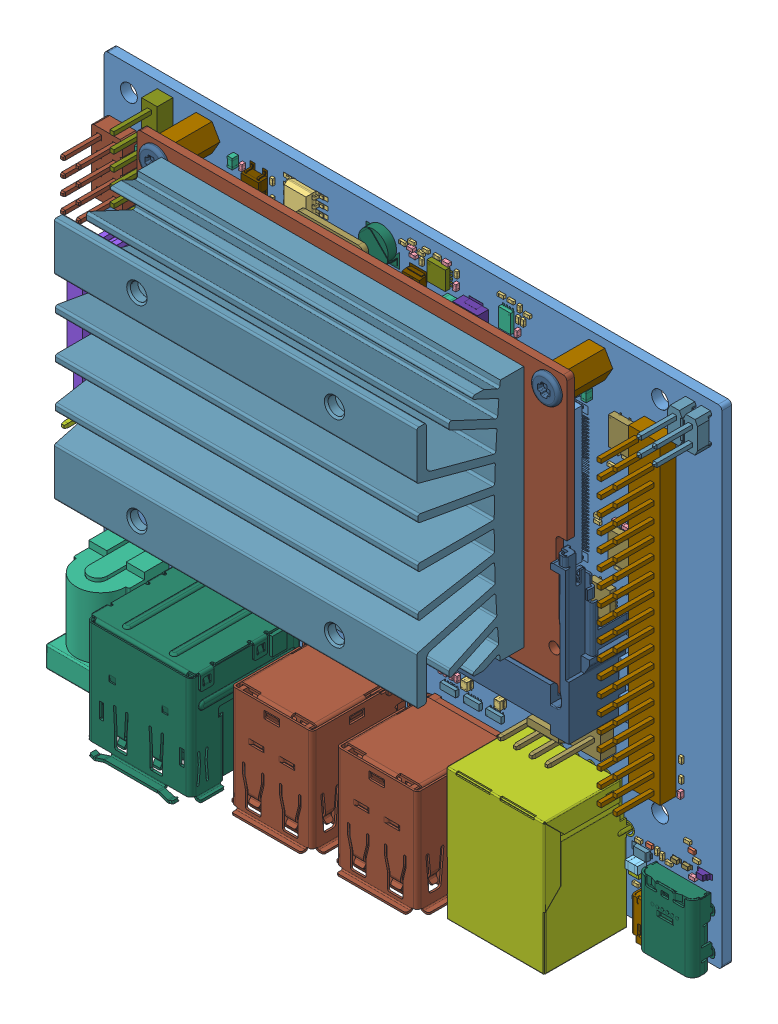
SolidWorks assembly P3450_P3449_A02_P3448_A02, configuration Valor predeterminado. Lengths in mm.
Overall size (100 81.03 30.51).
401 component instances, 71 part files, 0 mates.
Components (placement in the parent):
- 142-13449-1000-A02_ASM-1: 142-13449-1000-A02_ASM [Valor predeterminado] at origin size (100 81.03 23.18)
  - 142-13449-1000-A02-1: 142-13449-1000-A02 [Valor predeterminado] at origin size (100 79 1.57)
  - 315-1109-000_1-1: 315-1109-000_1 [Valor predeterminado] at (5.6 4.9 1.575) x (-1 0 0) z (0 0 1) size (4.5 3.5 0.8)
  - 0402_H040-1: 0402_H040 [Valor predeterminado] at (8 -0.825 1.575) size (1 0.5 0.4)
  - 0402_H060-1: 0402_H060 [Valor predeterminado] at (1 5 1.575) x (0 -1 0) z (0 0 1) size (1 0.5 0.6)
  - 0402_H040-2: 0402_H040 [Valor predeterminado] at (9.9 -0.3 1.575) size (1 0.5 0.4)
  - 0402_H040-3: 0402_H040 [Valor predeterminado] at (8.296 51.194 1.575) x (-1 0 0) z (0 0 1) size (1 0.5 0.4)
  - 0402_H040-4: 0402_H040 [Valor predeterminado] at (76.2 36.9 1.575) x (-1 0 0) z (0 0 1) size (1 0.5 0.4)
  - 0402_H040-5: 0402_H040 [Valor predeterminado] at (37.8 2.87 1.575) x (0 -1 0) z (0 0 1) size (1 0.5 0.4)
  - 0402_H040-6: 0402_H040 [Valor predeterminado] at (38.6 2.87 1.575) x (0 -1 0) z (0 0 1) size (1 0.5 0.4)
  - 0402_H060-2: 0402_H060 [Valor predeterminado] at (14.2 7.7 1.575) x (0 -1 0) z (0 0 1) size (1 0.5 0.6)
  - 0402_H040-7: 0402_H040 [Valor predeterminado] at (64 27.5 1.575) x (-1 0 0) z (0 0 1) size (1 0.5 0.4)
  - 0402_H060-3: 0402_H060 [Valor predeterminado] at (18.6 43.15 1.575) x (-1 0 0) z (0 0 1) size (1 0.5 0.6)
  - 0402_H060-4: 0402_H060 [Valor predeterminado] at (65.5 52.8 1.575) x (0 1 0) z (0 0 1) size (1 0.5 0.6)
  - 0402_H060-5: 0402_H060 [Valor predeterminado] at (64 28.4 1.575) x (-1 0 0) z (0 0 1) size (1 0.5 0.6)
  - 0402_H040-8: 0402_H040 [Valor predeterminado] at (60.95 25.85 1.575) size (1 0.5 0.4)
  - 0402_H060-6: 0402_H060 [Valor predeterminado] at (17.3 7.7 1.575) x (0 -1 0) z (0 0 1) size (1 0.5 0.6)
  - 0402_H060-7: 0402_H060 [Valor predeterminado] at (18.6 7.7 1.575) x (0 -1 0) z (0 0 1) size (1 0.5 0.6)
  - 0402_H060-8: 0402_H060 [Valor predeterminado] at (12.9 7.7 1.575) x (0 -1 0) z (0 0 1) size (1 0.5 0.6)
  - 0402_H060-9: 0402_H060 [Valor predeterminado] at (80.9 37.7 1.575) x (-1 0 0) z (0 0 1) size (1 0.5 0.6)
  - 0402_H040-9: 0402_H040 [Valor predeterminado] at (79.5 31.3 1.575) size (1 0.5 0.4)
  - 0402_H040-10: 0402_H040 [Valor predeterminado] at (81 31.3 1.575) x (-1 0 0) z (0 0 1) size (1 0.5 0.4)
  - 0402_H060-10: 0402_H060 [Valor predeterminado] at (79.3 37.7 1.575) size (1 0.5 0.6)
  - 0402_H060-11: 0402_H060 [Valor predeterminado] at (74.8 4.05 1.575) x (-1 0 0) z (0 0 1) size (1 0.5 0.6)
  - 0402_H040-11: 0402_H040 [Valor predeterminado] at (65.675 6.15 1.575) x (0 -1 0) z (0 0 1) size (1 0.5 0.4)
  - 0402_H060-12: 0402_H060 [Valor predeterminado] at (67.7 6.85 1.575) x (0 1 0) z (0 0 1) size (1 0.5 0.6)
  - 0402_H040-12: 0402_H040 [Valor predeterminado] at (64.475 5.8 1.575) x (-1 0 0) z (0 0 1) size (1 0.5 0.4)
  - 0402_H040-13: 0402_H040 [Valor predeterminado] at (67.725 5.325 1.575) x (0 1 0) z (0 0 1) size (1 0.5 0.4)
  - 0402_H060-13: 0402_H060 [Valor predeterminado] at (46.1 59.45 1.575) size (1 0.5 0.6)
  - 0402_H040-14: 0402_H040 [Valor predeterminado] at (44.65 59.45 1.575) size (1 0.5 0.4)
  - 0402_H040-15: 0402_H040 [Valor predeterminado] at (46.1 60.25 1.575) size (1 0.5 0.4)
  - 0402_H060-14: 0402_H060 [Valor predeterminado] at (53.35 57.7 1.575) x (0 -1 0) z (0 0 1) size (1 0.5 0.6)
  - 0402_H040-16: 0402_H040 [Valor predeterminado] at (47.6 59.45 1.575) size (1 0.5 0.4)
  - 0402_H040-17: 0402_H040 [Valor predeterminado] at (48.4 60.25 1.575) size (1 0.5 0.4)
  - 0402_H040-18: 0402_H040 [Valor predeterminado] at (47.7 58.325 1.575) x (0 1 0) z (0 0 1) size (1 0.5 0.4)
  - 0402_H060-15: 0402_H060 [Valor predeterminado] at (46.5 58.65 1.575) x (-1 0 0) z (0 0 1) size (1 0.5 0.6)
  - 0402_H060-16: 0402_H060 [Valor predeterminado] at (51.8 60.25 1.575) size (1 0.5 0.6)
  - 0402_H040-19: 0402_H040 [Valor predeterminado] at (53.35 59.4 1.575) x (0 -1 0) z (0 0 1) size (1 0.5 0.4)
  - 0402_H040-20: 0402_H040 [Valor predeterminado] at (50.2 60.25 1.575) x (-1 0 0) z (0 0 1) size (1 0.5 0.4)
  - 0402_H060-17: 0402_H060 [Valor predeterminado] at (18.6 43.95 1.575) x (-1 0 0) z (0 0 1) size (1 0.5 0.6)
  - 0402_H060-18: 0402_H060 [Valor predeterminado] at (52.75 2.9 1.575) x (0 -1 0) z (0 0 1) size (1 0.5 0.6)
  - 0402_H060-19: 0402_H060 [Valor predeterminado] at (22.35 47.4 1.575) x (-1 0 0) z (0 0 1) size (1 0.5 0.6)
  - 0402_H060-20: 0402_H060 [Valor predeterminado] at (20.55 47.4 1.575) x (-1 0 0) z (0 0 1) size (1 0.5 0.6)
  - 0402_H060-21: 0402_H060 [Valor predeterminado] at (21.95 34.55 1.575) x (0 -1 0) z (0 0 1) size (1 0.5 0.6)
  - 0402_H060-22: 0402_H060 [Valor predeterminado] at (21.05 34.55 1.575) x (0 -1 0) z (0 0 1) size (1 0.5 0.6)
  - 0402_H060-23: 0402_H060 [Valor predeterminado] at (53.55 2.9 1.575) x (0 -1 0) z (0 0 1) size (1 0.5 0.6)
  - 0402_H060-24: 0402_H060 [Valor predeterminado] at (25.4 54 1.575) x (-1 0 0) z (0 0 1) size (1 0.5 0.6)
  - 0402_H060-25: 0402_H060 [Valor predeterminado] at (24 34.58 1.575) x (0 -1 0) z (0 0 1) size (1 0.5 0.6)
  - 0402_H040-21: 0402_H040 [Valor predeterminado] at (55.6 2.95 1.575) x (0 -1 0) z (0 0 1) size (1 0.5 0.4)
  - 0402_H040-22: 0402_H040 [Valor predeterminado] at (20.13 34.53 1.575) x (0 1 0) z (0 0 1) size (1 0.5 0.4)
  - 0402_H060-26: 0402_H060 [Valor predeterminado] at (18.4 35.15 1.575) x (0 1 0) z (0 0 1) size (1 0.5 0.6)
  - 0402_H060-27: 0402_H060 [Valor predeterminado] at (18.4 36.75 1.575) x (0 1 0) z (0 0 1) size (1 0.5 0.6)
  - 0402_H040-23: 0402_H040 [Valor predeterminado] at (39.6 2.87 1.575) x (0 -1 0) z (0 0 1) size (1 0.5 0.4)
  - 0402_H040-24: 0402_H040 [Valor predeterminado] at (40.4 2.87 1.575) x (0 -1 0) z (0 0 1) size (1 0.5 0.4)
  - 0402_H040-25: 0402_H040 [Valor predeterminado] at (60.95 2.95 1.575) x (0 -1 0) z (0 0 1) size (1 0.5 0.4)
  - 0402_H040-26: 0402_H040 [Valor predeterminado] at (60.15 2.95 1.575) x (0 -1 0) z (0 0 1) size (1 0.5 0.4)
  - 0402_H040-27: 0402_H040 [Valor predeterminado] at (54.8 2.95 1.575) x (0 -1 0) z (0 0 1) size (1 0.5 0.4)
  - 0402_H040-28: 0402_H040 [Valor predeterminado] at (31.6 54 1.575) size (1 0.5 0.4)
  - 0402_H040-29: 0402_H040 [Valor predeterminado] at (27.4 54 1.575) size (1 0.5 0.4)
  - 0402_H040-30: 0402_H040 [Valor predeterminado] at (29.6 54 1.575) x (-1 0 0) z (0 0 1) size (1 0.5 0.4)
  - 0402_H040-31: 0402_H040 [Valor predeterminado] at (63.775 -14.475 1.575) size (1 0.5 0.4)
  - 0402_H040-32: 0402_H040 [Valor predeterminado] at (63.775 -15.275 1.575) size (1 0.5 0.4)
  - 0402_H040-33: 0402_H040 [Valor predeterminado] at (8.025 41.475 1.575) x (-1 0 0) z (0 0 1) size (1 0.5 0.4)
  - 0402_H060-28: 0402_H060 [Valor predeterminado] at (63.95 1.25 1.575) x (0 1 0) z (0 0 1) size (1 0.5 0.6)
  - 0402_H060-29: 0402_H060 [Valor predeterminado] at (2.95 54.05 1.575) x (0 1 0) z (0 0 1) size (1 0.5 0.6)
  - 0402_H040-34: 0402_H040 [Valor predeterminado] at (92.2 -3.45 1.575) x (-1 0 0) z (0 0 1) size (1 0.5 0.4)
  - 0402_H060-30: 0402_H060 [Valor predeterminado] at (32.85 7.7 1.575) x (0 -1 0) z (0 0 1) size (1 0.5 0.6)
  - 0402_H060-31: 0402_H060 [Valor predeterminado] at (27.25 7.7 1.575) x (0 -1 0) z (0 0 1) size (1 0.5 0.6)
  - 0402_H060-32: 0402_H060 [Valor predeterminado] at (31.25 7.7 1.575) x (0 -1 0) z (0 0 1) size (1 0.5 0.6)
  - 0402_H060-33: 0402_H060 [Valor predeterminado] at (28.85 7.7 1.575) x (0 -1 0) z (0 0 1) size (1 0.5 0.6)
  - 0402_H060-34: 0402_H060 [Valor predeterminado] at (32.05 7.7 1.575) x (0 -1 0) z (0 0 1) size (1 0.5 0.6)
  - 0402_H060-35: 0402_H060 [Valor predeterminado] at (28.05 7.7 1.575) x (0 -1 0) z (0 0 1) size (1 0.5 0.6)
  - 0402_H060-36: 0402_H060 [Valor predeterminado] at (30.45 7.7 1.575) x (0 -1 0) z (0 0 1) size (1 0.5 0.6)
  - 0402_H060-37: 0402_H060 [Valor predeterminado] at (29.65 7.7 1.575) x (0 -1 0) z (0 0 1) size (1 0.5 0.6)
  - 0402_H060-38: 0402_H060 [Valor predeterminado] at (24.65 6.41 1.575) x (0 -1 0) z (0 0 1) size (1 0.5 0.6)
  - 0402_H060-39: 0402_H060 [Valor predeterminado] at (25.85 6.41 1.575) x (0 -1 0) z (0 0 1) size (1 0.5 0.6)
  - 0402_H060-40: 0402_H060 [Valor predeterminado] at (4.2 36.5 1.575) x (0 1 0) z (0 0 1) size (1 0.5 0.6)
  - 0402_H060-41: 0402_H060 [Valor predeterminado] at (89.7 4.7 1.575) x (0 -1 0) z (0 0 1) size (1 0.5 0.6)
  - 0402_H060-42: 0402_H060 [Valor predeterminado] at (82.5 3.8 1.575) x (0 -1 0) z (0 0 1) size (1 0.5 0.6)
  - 0402_H060-43: 0402_H060 [Valor predeterminado] at (12.65 49.7 1.575) size (1 0.5 0.6)
  - 0402_H060-44: 0402_H060 [Valor predeterminado] at (11.2 50.15 1.575) x (0 -1 0) z (0 0 1) size (1 0.5 0.6)
  - 0402_H060-45: 0402_H060 [Valor predeterminado] at (26.5 34.55 1.575) x (0 -1 0) z (0 0 1) size (1 0.5 0.6)
  - 0402_H060-46: 0402_H060 [Valor predeterminado] at (29.9 34.5 1.575) x (0 -1 0) z (0 0 1) size (1 0.5 0.6)
  - 0402_H060-47: 0402_H060 [Valor predeterminado] at (31.7 40.15 1.575) x (0 1 0) z (0 0 1) size (1 0.5 0.6)
  - 0402_H060-48: 0402_H060 [Valor predeterminado] at (31.15 42.5 1.575) x (0 1 0) z (0 0 1) size (1 0.5 0.6)
  - 0402_H060-49: 0402_H060 [Valor predeterminado] at (19.2 47.05 1.575) x (0 1 0) z (0 0 1) size (1 0.5 0.6)
  - 0402_H060-50: 0402_H060 [Valor predeterminado] at (17.95 42 1.575) x (0 -1 0) z (0 0 1) size (1 0.5 0.6)
  - 0402_H060-51: 0402_H060 [Valor predeterminado] at (27.3 48.25 1.575) x (0 1 0) z (0 0 1) size (1 0.5 0.6)
  - 0402_H060-52: 0402_H060 [Valor predeterminado] at (31.7 37.85 1.575) x (0 -1 0) z (0 0 1) size (1 0.5 0.6)
  - 0402_H060-53: 0402_H060 [Valor predeterminado] at (29.6 48.35 1.575) x (0 1 0) z (0 0 1) size (1 0.5 0.6)
  - 0402_H060-54: 0402_H060 [Valor predeterminado] at (18.8 38.75 1.575) x (-1 0 0) z (0 0 1) size (1 0.5 0.6)
  - 0402_H060-55: 0402_H060 [Valor predeterminado] at (18.7 57.2 1.575) x (0 -1 0) z (0 0 1) size (1 0.5 0.6)
  - 0402_H060-56: 0402_H060 [Valor predeterminado] at (34.1 2.9 1.575) x (0 -1 0) z (0 0 1) size (1 0.5 0.6)
  - 0402_H060-57: 0402_H060 [Valor predeterminado] at (35.8 2.9 1.575) x (0 -1 0) z (0 0 1) size (1 0.5 0.6)
  - 0402_H060-58: 0402_H060 [Valor predeterminado] at (34.9 2.9 1.575) x (0 -1 0) z (0 0 1) size (1 0.5 0.6)
  - 0402_H060-59: 0402_H060 [Valor predeterminado] at (36.6 2.9 1.575) x (0 -1 0) z (0 0 1) size (1 0.5 0.6)
  - 0402_H060-60: 0402_H060 [Valor predeterminado] at (11.325 44.725 1.575) size (1 0.5 0.6)
  - 0402_H060-61: 0402_H060 [Valor predeterminado] at (50.95 2.9 1.575) x (0 -1 0) z (0 0 1) size (1 0.5 0.6)
  - 0402_H060-62: 0402_H060 [Valor predeterminado] at (51.75 2.9 1.575) x (0 -1 0) z (0 0 1) size (1 0.5 0.6)
  - 0402_H060-63: 0402_H060 [Valor predeterminado] at (11.55 39.7 1.575) size (1 0.5 0.6)
  - 0402_H060-64: 0402_H060 [Valor predeterminado] at (9.5 -8.5 1.575) x (-1 0 0) z (0 0 1) size (1 0.5 0.6)
  - 0402_H060-65: 0402_H060 [Valor predeterminado] at (61.35 38.05 1.575) x (0 -1 0) z (0 0 1) size (1 0.5 0.6)
  - 0402_H060-66: 0402_H060 [Valor predeterminado] at (60.55 38.05 1.575) x (0 -1 0) z (0 0 1) size (1 0.5 0.6)
  - 0402_H060-67: 0402_H060 [Valor predeterminado] at (29.3 25.65 1.575) x (0 -1 0) z (0 0 1) size (1 0.5 0.6)
  - 0402_H060-68: 0402_H060 [Valor predeterminado] at (63.3 56.2 1.575) x (0 1 0) z (0 0 1) size (1 0.5 0.6)
  - 0402_H060-69: 0402_H060 [Valor predeterminado] at (20.5 54.2 1.575) size (1 0.5 0.6)
  - 0402_H060-70: 0402_H060 [Valor predeterminado] at (60.1 32.15 1.575) x (0 1 0) z (0 0 1) size (1 0.5 0.6)
  - 0402_H060-71: 0402_H060 [Valor predeterminado] at (60.9 32.15 1.575) x (0 1 0) z (0 0 1) size (1 0.5 0.6)
  - 0402_H060-72: 0402_H060 [Valor predeterminado] at (18.6 44.85 1.575) size (1 0.5 0.6)
  - 0402_H060-73: 0402_H060 [Valor predeterminado] at (18.6 45.65 1.575) size (1 0.5 0.6)
  - 0402_H060-74: 0402_H060 [Valor predeterminado] at (18.1 27.25 1.575) size (1 0.5 0.6)
  - 0402_H060-75: 0402_H060 [Valor predeterminado] at (15.1 7.7 1.575) x (0 -1 0) z (0 0 1) size (1 0.5 0.6)
  - 0402_H060-76: 0402_H060 [Valor predeterminado] at (16.4 7.7 1.575) x (0 -1 0) z (0 0 1) size (1 0.5 0.6)
  - 0402_H060-77: 0402_H060 [Valor predeterminado] at (20.8 7.7 1.575) x (0 -1 0) z (0 0 1) size (1 0.5 0.6)
  - 0402_H060-78: 0402_H060 [Valor predeterminado] at (19.5 7.7 1.575) x (0 -1 0) z (0 0 1) size (1 0.5 0.6)
  - 0402_H060-79: 0402_H060 [Valor predeterminado] at (21.9 2.8 1.575) size (1 0.5 0.6)
  - 0402_H060-80: 0402_H060 [Valor predeterminado] at (12.75 29 1.575) size (1 0.5 0.6)
  - 0402_H060-81: 0402_H060 [Valor predeterminado] at (10.225 5.1 1.575) size (1 0.5 0.6)
  - 0402_H060-82: 0402_H060 [Valor predeterminado] at (22.8 27.65 1.575) x (0 1 0) z (0 0 1) size (1 0.5 0.6)
  - 0402_H060-83: 0402_H060 [Valor predeterminado] at (18.85 25.15 1.575) x (0 -1 0) z (0 0 1) size (1 0.5 0.6)
  - 0402_H060-84: 0402_H060 [Valor predeterminado] at (17.95 40.1 1.575) x (0 1 0) z (0 0 1) size (1 0.5 0.6)
  - 0402_H040-35: 0402_H040 [Valor predeterminado] at (20.8 6.2 1.575) x (0 1 0) z (0 0 1) size (1 0.5 0.4)
  - 0402_H040-36: 0402_H040 [Valor predeterminado] at (76 22.7 1.575) size (1 0.5 0.4)
  - 0402_H040-37: 0402_H040 [Valor predeterminado] at (23.7 26.85 1.575) x (0 1 0) z (0 0 1) size (1 0.5 0.4)
  - 0402_H040-38: 0402_H040 [Valor predeterminado] at (18 25.15 1.575) x (0 1 0) z (0 0 1) size (1 0.5 0.4)
  - 0402_H040-39: 0402_H040 [Valor predeterminado] at (17.3 28.25 1.575) x (-1 0 0) z (0 0 1) size (1 0.5 0.4)
  - 0402_H040-40: 0402_H040 [Valor predeterminado] at (13.15 4.2 1.575) x (0 -1 0) z (0 0 1) size (1 0.5 0.4)
  - 0402_H040-41: 0402_H040 [Valor predeterminado] at (17.2 30.15 1.575) x (0 -1 0) z (0 0 1) size (1 0.5 0.4)
  - 0402_H040-42: 0402_H040 [Valor predeterminado] at (14.2 6.2 1.575) x (0 1 0) z (0 0 1) size (1 0.5 0.4)
  - 0402_H040-43: 0402_H040 [Valor predeterminado] at (12.9 6.2 1.575) x (0 1 0) z (0 0 1) size (1 0.5 0.4)
  - 0402_H040-44: 0402_H040 [Valor predeterminado] at (15.1 6.2 1.575) x (0 1 0) z (0 0 1) size (1 0.5 0.4)
  - 0402_H040-45: 0402_H040 [Valor predeterminado] at (16.4 6.2 1.575) x (0 1 0) z (0 0 1) size (1 0.5 0.4)
  - 0402_H040-46: 0402_H040 [Valor predeterminado] at (19.5 6.2 1.575) x (0 1 0) z (0 0 1) size (1 0.5 0.4)
  - 0402_H040-47: 0402_H040 [Valor predeterminado] at (17.3 6.2 1.575) x (0 1 0) z (0 0 1) size (1 0.5 0.4)
  - 0402_H040-48: 0402_H040 [Valor predeterminado] at (18.6 6.2 1.575) x (0 1 0) z (0 0 1) size (1 0.5 0.4)
  - 0402_H040-49: 0402_H040 [Valor predeterminado] at (24.2 24.55 1.575) x (0 1 0) z (0 0 1) size (1 0.5 0.4)
  - 0402_H040-50: 0402_H040 [Valor predeterminado] at (23.5 54.9 1.575) x (0 1 0) z (0 0 1) size (1 0.5 0.4)
  - 0402_H040-51: 0402_H040 [Valor predeterminado] at (13.2 39.75 1.575) x (-1 0 0) z (0 0 1) size (1 0.5 0.4)
  - 0402_H040-52: 0402_H040 [Valor predeterminado] at (80.7 47.4 1.575) x (-1 0 0) z (0 0 1) size (1 0.5 0.4)
  - 0402_H040-53: 0402_H040 [Valor predeterminado] at (77.5 22.7 1.575) x (-1 0 0) z (0 0 1) size (1 0.5 0.4)
  - 0402_H040-54: 0402_H040 [Valor predeterminado] at (9.25 -12.75 1.575) x (-1 0 0) z (0 0 1) size (1 0.5 0.4)
  - 0402_H040-55: 0402_H040 [Valor predeterminado] at (9.25 -11.95 1.575) x (-1 0 0) z (0 0 1) size (1 0.5 0.4)
  - 0402_H040-56: 0402_H040 [Valor predeterminado] at (64.475 6.7 1.575) size (1 0.5 0.4)
  - 0402_H040-57: 0402_H040 [Valor predeterminado] at (29.3 24 1.575) x (0 1 0) z (0 0 1) size (1 0.5 0.4)
  - 0402_H040-58: 0402_H040 [Valor predeterminado] at (64.2 32.5 1.575) x (0 1 0) z (0 0 1) size (1 0.5 0.4)
  - 0402_H040-59: 0402_H040 [Valor predeterminado] at (64.15 47.45 1.575) x (0 -1 0) z (0 0 1) size (1 0.5 0.4)
  - 0402_H040-60: 0402_H040 [Valor predeterminado] at (64.2 31 1.575) x (0 -1 0) z (0 0 1) size (1 0.5 0.4)
  - 0402_H040-61: 0402_H040 [Valor predeterminado] at (76.2 36.1 1.575) x (-1 0 0) z (0 0 1) size (1 0.5 0.4)
  - 0402_H040-62: 0402_H040 [Valor predeterminado] at (78.4 45.15 1.575) size (1 0.5 0.4)
  - 0402_H040-63: 0402_H040 [Valor predeterminado] at (81.7 38.6 1.575) size (1 0.5 0.4)
  - 0402_H040-64: 0402_H040 [Valor predeterminado] at (81.7 39.4 1.575) size (1 0.5 0.4)
  - 0402_H040-65: 0402_H040 [Valor predeterminado] at (59.35 51.825 1.575) size (1 0.5 0.4)
  - 0402_H040-66: 0402_H040 [Valor predeterminado] at (60.825 51.825 1.575) x (-1 0 0) z (0 0 1) size (1 0.5 0.4)
  - 0402_H040-67: 0402_H040 [Valor predeterminado] at (89.7 9.5 1.575) x (0 1 0) z (0 0 1) size (1 0.5 0.4)
  - 0402_H040-68: 0402_H040 [Valor predeterminado] at (89.7 6.7 1.575) x (0 1 0) z (0 0 1) size (1 0.5 0.4)
  - 0402_H040-69: 0402_H040 [Valor predeterminado] at (3.9 34.2 1.575) x (0 -1 0) z (0 0 1) size (1 0.5 0.4)
  - 0402_H040-70: 0402_H040 [Valor predeterminado] at (5.1 35 1.575) x (0 1 0) z (0 0 1) size (1 0.5 0.4)
  - 0402_H040-71: 0402_H040 [Valor predeterminado] at (32.85 5.81 1.575) x (0 -1 0) z (0 0 1) size (1 0.5 0.4)
  - 0402_H040-72: 0402_H040 [Valor predeterminado] at (32.05 5.81 1.575) x (0 -1 0) z (0 0 1) size (1 0.5 0.4)
  - 0402_H040-73: 0402_H040 [Valor predeterminado] at (27.25 5.81 1.575) x (0 -1 0) z (0 0 1) size (1 0.5 0.4)
  - 0402_H040-74: 0402_H040 [Valor predeterminado] at (28.05 5.81 1.575) x (0 -1 0) z (0 0 1) size (1 0.5 0.4)
  - 0402_H040-75: 0402_H040 [Valor predeterminado] at (31.25 5.81 1.575) x (0 -1 0) z (0 0 1) size (1 0.5 0.4)
  - 0402_H040-76: 0402_H040 [Valor predeterminado] at (30.45 5.81 1.575) x (0 -1 0) z (0 0 1) size (1 0.5 0.4)
  - 0402_H040-77: 0402_H040 [Valor predeterminado] at (28.85 5.81 1.575) x (0 -1 0) z (0 0 1) size (1 0.5 0.4)
  - 0402_H040-78: 0402_H040 [Valor predeterminado] at (29.65 5.81 1.575) x (0 -1 0) z (0 0 1) size (1 0.5 0.4)
  - 0402_H040-79: 0402_H040 [Valor predeterminado] at (13.5 52.9 1.575) x (-1 0 0) z (0 0 1) size (1 0.5 0.4)
  - 0402_H040-80: 0402_H040 [Valor predeterminado] at (22.35 4 1.575) x (0 -1 0) z (0 0 1) size (1 0.5 0.4)
  - 0402_H040-81: 0402_H040 [Valor predeterminado] at (21.55 4 1.575) x (0 1 0) z (0 0 1) size (1 0.5 0.4)
  - 0402_H040-82: 0402_H040 [Valor predeterminado] at (25.85 4.9 1.575) x (0 -1 0) z (0 0 1) size (1 0.5 0.4)
  - 0402_H040-83: 0402_H040 [Valor predeterminado] at (11.8 52.9 1.575) size (1 0.5 0.4)
  - 0402_H040-84: 0402_H040 [Valor predeterminado] at (9.432 51.594 1.575) x (0 -1 0) z (0 0 1) size (1 0.5 0.4)
  - 0402_H040-85: 0402_H040 [Valor predeterminado] at (8.975 50.3 1.575) size (1 0.5 0.4)
  - 0402_H040-86: 0402_H040 [Valor predeterminado] at (82.8 -5.3 1.575) x (-1 0 0) z (0 0 1) size (1 0.5 0.4)
  - 0402_H040-87: 0402_H040 [Valor predeterminado] at (82.4 -11.6 1.575) x (-1 0 0) z (0 0 1) size (1 0.5 0.4)
  - 0402_H040-88: 0402_H040 [Valor predeterminado] at (22.8 26.05 1.575) x (0 1 0) z (0 0 1) size (1 0.5 0.4)
  - 0402_H040-89: 0402_H040 [Valor predeterminado] at (20.8 28.25 1.575) size (1 0.5 0.4)
  - 0402_H040-90: 0402_H040 [Valor predeterminado] at (20.8 24.65 1.575) x (-1 0 0) z (0 0 1) size (1 0.5 0.4)
  - 0402_H040-91: 0402_H040 [Valor predeterminado] at (18.1 26.45 1.575) size (1 0.5 0.4)
  - 0402_H040-92: 0402_H040 [Valor predeterminado] at (24.65 8.41 1.575) x (0 1 0) z (0 0 1) size (1 0.5 0.4)
  - 0402_H040-93: 0402_H040 [Valor predeterminado] at (25.85 8.41 1.575) x (0 1 0) z (0 0 1) size (1 0.5 0.4)
  - 0402_H040-94: 0402_H040 [Valor predeterminado] at (3.8 54.4 1.575) x (0 -1 0) z (0 0 1) size (1 0.5 0.4)
  - 0402_H040-95: 0402_H040 [Valor predeterminado] at (2.45 44.45 1.575) x (0 -1 0) z (0 0 1) size (1 0.5 0.4)
  - 0402_H040-96: 0402_H040 [Valor predeterminado] at (24.65 4.9 1.575) x (0 1 0) z (0 0 1) size (1 0.5 0.4)
  - 0402_H040-97: 0402_H040 [Valor predeterminado] at (22.15 7.6 1.575) x (-1 0 0) z (0 0 1) size (1 0.5 0.4)
  - 0402_H040-98: 0402_H040 [Valor predeterminado] at (79.2 47.4 1.575) size (1 0.5 0.4)
  - 0402_H040-99: 0402_H040 [Valor predeterminado] at (19 28.25 1.575) size (1 0.5 0.4)
  - 0402_H040-100: 0402_H040 [Valor predeterminado] at (9.65 9.7 1.575) x (0 -1 0) z (0 0 1) size (1 0.5 0.4)
  - 0402_H040-101: 0402_H040 [Valor predeterminado] at (28.35 34.45 1.575) x (0 1 0) z (0 0 1) size (1 0.5 0.4)
  - 0402_H040-102: 0402_H040 [Valor predeterminado] at (25.2 34.55 1.575) x (0 1 0) z (0 0 1) size (1 0.5 0.4)
  - 0402_H040-103: 0402_H040 [Valor predeterminado] at (10.625 6.35 1.575) x (0 -1 0) z (0 0 1) size (1 0.5 0.4)
  - 0402_H040-104: 0402_H040 [Valor predeterminado] at (9.825 6.35 1.575) x (0 1 0) z (0 0 1) size (1 0.5 0.4)
  - 0402_H040-105: 0402_H040 [Valor predeterminado] at (4.775 42.975 1.575) x (0 1 0) z (0 0 1) size (1 0.5 0.4)
  - 0402_H040-106: 0402_H040 [Valor predeterminado] at (19.8 32.9 1.575) x (-1 0 0) z (0 0 1) size (1 0.5 0.4)
  - 0402_H040-107: 0402_H040 [Valor predeterminado] at (22.35 24.65 1.575) x (-1 0 0) z (0 0 1) size (1 0.5 0.4)
  - 0402_H040-108: 0402_H040 [Valor predeterminado] at (62.4 54.7 1.575) size (1 0.5 0.4)
  - 0402_H040-109: 0402_H040 [Valor predeterminado] at (62.2 60.05 1.575) x (-1 0 0) z (0 0 1) size (1 0.5 0.4)
  - 0402_H040-110: 0402_H040 [Valor predeterminado] at (23.5 57.5 1.575) x (0 1 0) z (0 0 1) size (1 0.5 0.4)
  - 0402_H040-111: 0402_H040 [Valor predeterminado] at (12.8 44.725 1.575) size (1 0.5 0.4)
  - 0402_H040-112: 0402_H040 [Valor predeterminado] at (21.8 31.45 1.575) x (0 1 0) z (0 0 1) size (1 0.5 0.4)
  - 0402_H040-113: 0402_H040 [Valor predeterminado] at (19.25 34.55 1.575) x (0 1 0) z (0 0 1) size (1 0.5 0.4)
  - 0402_H040-114: 0402_H040 [Valor predeterminado] at (0.95 41.55 1.575) size (1 0.5 0.4)
  - 0402_H040-115: 0402_H040 [Valor predeterminado] at (64.1 58 1.575) x (0 1 0) z (0 0 1) size (1 0.5 0.4)
  - 0402_H040-116: 0402_H040 [Valor predeterminado] at (63.3 58 1.575) x (0 -1 0) z (0 0 1) size (1 0.5 0.4)
  - 0402_H040-117: 0402_H040 [Valor predeterminado] at (63.55 59.7 1.575) x (0 -1 0) z (0 0 1) size (1 0.5 0.4)
  - 0402_H060-85: 0402_H060 [Valor predeterminado] at (71.175 4 1.575) x (-1 0 0) z (0 0 1) size (1 0.5 0.6)
  - 0402_H040-118: 0402_H040 [Valor predeterminado] at (86.6 -5.6 1.575) x (0 1 0) z (0 0 1) size (1 0.5 0.4)
  - 0402_H040-119: 0402_H040 [Valor predeterminado] at (85.8 -5.3 1.575) x (0 1 0) z (0 0 1) size (1 0.5 0.4)
  - 0402_H040-120: 0402_H040 [Valor predeterminado] at (10.25 51.6 1.575) x (0 1 0) z (0 0 1) size (1 0.5 0.4)
  - 0402_H040-121: 0402_H040 [Valor predeterminado] at (80.5 28.55 1.575) size (1 0.5 0.4)
  - 0402_H040-122: 0402_H040 [Valor predeterminado] at (13.95 4.2 1.575) x (0 -1 0) z (0 0 1) size (1 0.5 0.4)
  - 0402_H040-123: 0402_H040 [Valor predeterminado] at (15.35 4.2 1.575) x (0 -1 0) z (0 0 1) size (1 0.5 0.4)
  - 0402_H040-124: 0402_H040 [Valor predeterminado] at (16.15 4.2 1.575) x (0 -1 0) z (0 0 1) size (1 0.5 0.4)
  - 0402_H040-125: 0402_H040 [Valor predeterminado] at (20.55 4.2 1.575) x (0 -1 0) z (0 0 1) size (1 0.5 0.4)
  - 0402_H040-126: 0402_H040 [Valor predeterminado] at (19.75 4.2 1.575) x (0 -1 0) z (0 0 1) size (1 0.5 0.4)
  - 0402_H040-127: 0402_H040 [Valor predeterminado] at (17.6 4.2 1.575) x (0 -1 0) z (0 0 1) size (1 0.5 0.4)
  - 0402_H040-128: 0402_H040 [Valor predeterminado] at (18.4 4.2 1.575) x (0 -1 0) z (0 0 1) size (1 0.5 0.4)
  - 0402_H060-86: 0402_H060 [Valor predeterminado] at (64.25 -13.325 1.575) x (0 -1 0) z (0 0 1) size (1 0.5 0.6)
  - 0402_H060-87: 0402_H060 [Valor predeterminado] at (64.225 -11.825 1.575) x (0 1 0) z (0 0 1) size (1 0.5 0.6)
  - 0402_H040-129: 0402_H040 [Valor predeterminado] at (63.8 -6.85 1.575) x (0 1 0) z (0 0 1) size (1 0.5 0.4)
  - 0402_H040-130: 0402_H040 [Valor predeterminado] at (81.7 41.95 1.575) size (1 0.5 0.4)
  - 0402_H040-131: 0402_H040 [Valor predeterminado] at (87.75 -6 1.575) x (-1 0 0) z (0 0 1) size (1 0.5 0.4)
  - 0402_H040-132: 0402_H040 [Valor predeterminado] at (82.4 -13.6 1.575) x (-1 0 0) z (0 0 1) size (1 0.5 0.4)
  - 0402_H060-88: 0402_H060 [Valor predeterminado] at (91.75 -5.95 1.575) size (1 0.5 0.6)
  - 0402_H040-133: 0402_H040 [Valor predeterminado] at (3.65 49.25 1.575) x (0 -1 0) z (0 0 1) size (1 0.5 0.4)
  - 0402_H040-134: 0402_H040 [Valor predeterminado] at (2.45 49.25 1.575) x (0 1 0) z (0 0 1) size (1 0.5 0.4)
  - 0402_H040-135: 0402_H040 [Valor predeterminado] at (90.75 -1.45 1.575) x (-1 0 0) z (0 0 1) size (1 0.5 0.4)
  - 0402_H040-136: 0402_H040 [Valor predeterminado] at (8.45 39.55 1.575) x (0 -1 0) z (0 0 1) size (1 0.5 0.4)
  - 0402_H060-89: 0402_H060 [Valor predeterminado] at (8.85 -5.25 1.575) x (-1 0 0) z (0 0 1) size (1 0.5 0.6)
  - 0402_H040-137: 0402_H040 [Valor predeterminado] at (18.6 32.55 1.575) x (0 1 0) z (0 0 1) size (1 0.5 0.4)
  - 0402_H060-90: 0402_H060 [Valor predeterminado] at (4.5 44.45 1.575) x (0 1 0) z (0 0 1) size (1 0.5 0.6)
  - 0402_H040-138: 0402_H040 [Valor predeterminado] at (8.35 2.75 1.575) size (1 0.5 0.4)
  - 0402_H040-139: 0402_H040 [Valor predeterminado] at (9.4 1.95 1.575) size (1 0.5 0.4)
  - 0402_H040-140: 0402_H040 [Valor predeterminado] at (8.2 1.55 1.575) x (0 1 0) z (0 0 1) size (1 0.5 0.4)
  - 0402_H060-91: 0402_H060 [Valor predeterminado] at (8.5 3.875 1.575) x (0 -1 0) z (0 0 1) size (1 0.5 0.6)
  - 0402_H060-92: 0402_H060 [Valor predeterminado] at (-0.8 41.5 1.575) x (-1 0 0) z (0 0 1) size (1 0.5 0.6)
  - 0402_H040-141: 0402_H040 [Valor predeterminado] at (-1.35 7.75 1.575) size (1 0.5 0.4)
  - 0402_H040-142: 0402_H040 [Valor predeterminado] at (8 0.425 1.575) size (1 0.5 0.4)
  - 0402_H040-143: 0402_H040 [Valor predeterminado] at (67.9 4.025 1.575) x (-1 0 0) z (0 0 1) size (1 0.5 0.4)
  - 0402_H040-144: 0402_H040 [Valor predeterminado] at (60.6 60.05 1.575) x (-1 0 0) z (0 0 1) size (1 0.5 0.4)
  - 0402_H040-145: 0402_H040 [Valor predeterminado] at (72.85 4 1.575) x (-1 0 0) z (0 0 1) size (1 0.5 0.4)
  - 0402_H040-146: 0402_H040 [Valor predeterminado] at (64.8 59.35 1.575) size (1 0.5 0.4)
  - 0402_H040-147: 0402_H040 [Valor predeterminado] at (7.2 7.3 1.575) size (1 0.5 0.4)
  - 0402_H040-148: 0402_H040 [Valor predeterminado] at (8.5 5.35 1.575) x (0 1 0) z (0 0 1) size (1 0.5 0.4)
  - 0402_H040-149: 0402_H040 [Valor predeterminado] at (8.475 7.075 1.575) x (0 1 0) z (0 0 1) size (1 0.5 0.4)
  - VIRTUAL_SHORT-1: VIRTUAL_SHORT [Valor predeterminado] at (23.5 32.9 1.575) x (0 1 0) z (0 0 1) size (0.25 0.25 1)
  - VIRTUAL_SHORT-2: VIRTUAL_SHORT [Valor predeterminado] at (26.85 32.85 1.575) x (0 1 0) z (0 0 1) size (0.25 0.25 1)
  - VIRTUAL_SHORT-3: VIRTUAL_SHORT [Valor predeterminado] at (30.6 33.8 1.575) x (0 1 0) z (0 0 1) size (0.25 0.25 1)
  - VIRTUAL_SHORT-4: VIRTUAL_SHORT [Valor predeterminado] at (32.65 39.75 1.575) x (-1 0 0) z (0 0 1) size (0.25 0.25 1)
  - VIRTUAL_SHORT-5: VIRTUAL_SHORT [Valor predeterminado] at (31.85 42.1 1.575) x (-1 0 0) z (0 0 1) size (0.25 0.25 1)
  - VIRTUAL_SHORT-6: VIRTUAL_SHORT [Valor predeterminado] at (17.35 42.4 1.575) size (0.25 0.25 1)
  - VIRTUAL_SHORT-7: VIRTUAL_SHORT [Valor predeterminado] at (18.6 46.6 1.575) size (0.25 0.25 1)
  - VIRTUAL_SHORT-8: VIRTUAL_SHORT [Valor predeterminado] at (20.9 32.9 1.575) x (0 1 0) z (0 0 1) size (0.25 0.25 1)
  - VIRTUAL_SHORT-9: VIRTUAL_SHORT [Valor predeterminado] at (28.6 48.25 1.575) x (0 -1 0) z (0 0 1) size (0.25 0.25 1)
  - VIRTUAL_SHORT-10: VIRTUAL_SHORT [Valor predeterminado] at (27.1 49.35 1.575) x (0 -1 0) z (0 0 1) size (0.25 0.25 1)
  - VIRTUAL_SHORT-11: VIRTUAL_SHORT [Valor predeterminado] at (22.1 32.95 1.575) x (-1 0 0) z (0 0 1) size (0.25 0.25 1)
  - VIRTUAL_SHORT-12: VIRTUAL_SHORT [Valor predeterminado] at (32.65 38.25 1.575) x (-1 0 0) z (0 0 1) size (0.25 0.25 1)
  - VIRTUAL_SHORT-13: VIRTUAL_SHORT [Valor predeterminado] at (30.3 48 1.575) x (-1 0 0) z (0 0 1) size (0.25 0.25 1)
  - VIRTUAL_SHORT-14: VIRTUAL_SHORT [Valor predeterminado] at (17.15 38.95 1.575) size (0.25 0.25 1)
  - VIRTUAL_SHORT-15: VIRTUAL_SHORT [Valor predeterminado] at (17.15 39.7 1.575) size (0.25 0.25 1)
  - VIRTUAL_SHORT-16: VIRTUAL_SHORT [Valor predeterminado] at (76.175 4.1 1.575) x (-1 0 0) z (0 0 1) size (0.25 0.25 1)
  - 064-0377-000_2-1: 064-0377-000_2 [Valor predeterminado] at (2 -4.75 1.575) x (0 -1 0) z (0 0 1) size (14.63 10.08 14.5)
  - 074-0117-000_2-1: 074-0117-000_2 [Valor predeterminado] at (0.254 14.3 1.575) size (5.08 2.54 11.66)
  - 090-0096-000_1-1: 090-0096-000_1 [Valor predeterminado] at (3.45 44.4 1.575) x (0 -1 0) z (0 0 1) size (1.2 0.6 0.4)
  - 090-0309-000_1-1: 090-0309-000_1 [Valor predeterminado] at (-1.65 8.7 1.575) x (-1 0 0) z (0 0 1) size (1.2 0.6 0.4)
  - 115-1232-000_2-1: 115-1232-000_2 [Valor predeterminado] at (1.25 6.5 1.575) x (-1 0 0) z (0 0 1) size (0.9 0.9 0.33)
  - 074-0102-000_4-1: 074-0102-000_4 [Valor predeterminado] at (0.254 44.36 1.575) x (0 1 0) z (0 0 1) size (10.16 5.08 11.6)
  - 064-0400-000_1-1: 064-0400-000_1 [Valor predeterminado] at (73.75 7.77 1.575) size (10.16 5.8 13.5)
  - MEC_STANDOFF_PTH_620C380P-1: MEC_STANDOFF_PTH_620C380P [Valor predeterminado] at (40.276 40.3 1.575) x (0 1 0) z (0 0 1) size (6.2 6.2 0.73)
  - 090-0231-000_1-1: 090-0231-000_1 [Valor predeterminado] at (35.3 0.7 1.575) x (-1 0 0) z (0 0 1) size (2.5 1.55 0.55)
  - 090-0231-000_1-2: 090-0231-000_1 [Valor predeterminado] at (52.25 0.7 1.575) x (-1 0 0) z (0 0 1) size (2.5 1.55 0.55)
  - 090-0231-000_1-3: 090-0231-000_1 [Valor predeterminado] at (56.05 0.7 1.575) size (2.5 1.55 0.55)
  - 090-0231-000_1-4: 090-0231-000_1 [Valor predeterminado] at (59.65 0.7 1.575) size (2.5 1.55 0.55)
  - 090-0231-000_1-5: 090-0231-000_1 [Valor predeterminado] at (39.1 0.7 1.575) size (2.5 1.55 0.55)
  - 090-0231-000_1-6: 090-0231-000_1 [Valor predeterminado] at (43.1 0.7 1.575) size (2.5 1.55 0.55)
  - 090-0231-000_1-7: 090-0231-000_1 [Valor predeterminado] at (14.6 1.8 1.575) size (2.5 1.55 0.55)
  - 090-0231-000_1-8: 090-0231-000_1 [Valor predeterminado] at (19.1 1.8 1.575) size (2.5 1.55 0.55)
  - 090-0231-000_1-9: 090-0231-000_1 [Valor predeterminado] at (22.5 1.4 1.575) size (2.5 1.55 0.55)
  - 090-0231-000_1-10: 090-0231-000_1 [Valor predeterminado] at (28.45 3.35 1.575) size (2.5 1.55 0.55)
  - 090-0231-000_1-11: 090-0231-000_1 [Valor predeterminado] at (31.65 3.35 1.575) size (2.5 1.55 0.55)
  - 064-0305-000_2-1: 064-0305-000_2 [Valor predeterminado] at (90 -12.2 1.575) size (9.87 10.86 4.08)
  - 074-0223-000_2-1: 074-0223-000_2 [Valor predeterminado] at (5.85 53.25 1.575) x (0 1 0) z (0 0 1) size (15.24 2.54 11.6)
  - 131-0832-000_2-1: 131-0832-000_2 [Valor predeterminado] at (56.3 54.7 1.575) x (0 -1 0) z (0 0 1) size (4.96 4.06 1.8)
  - 115-0836-000_1-1: 115-0836-000_1 [Valor predeterminado] at (21.1 56.6 1.575) size (2.9 3.58 1.45)
  - 115-0836-000_1-2: 115-0836-000_1 [Valor predeterminado] at (11.8 42.3 1.575) size (2.9 3.58 1.45)
  - 315-0620-000_1-1: 315-0620-000_1 [Valor predeterminado] at (72.1 53.4 1.575) x (0 -1 0) z (0 0 1) size (2.9 3.58 1.1)
  - 315-1062-000_1-1: 315-1062-000_1 [Valor predeterminado] at (26.8 25.15 1.575) x (0 -1 0) z (0 0 1) size (2.9 3.58 1.45)
  - 170-0285-000_1-1: 170-0285-000_1 [Valor predeterminado] at (28.72 57.28 1.575) x (0 1 0) z (0 0 1) size (4.9 7.21 1.75)
  - 115-0138-000_1-1: 115-0138-000_1 [Valor predeterminado] at (9.15 48.55 1.575) x (0 1 0) z (0 0 1) size (2 2.88 1.1)
  - 115-1821-000_1-1: 115-1821-000_1 [Valor predeterminado] at (3.3 40.8 1.575) x (-1 0 0) z (0 0 1) size (2 2.88 1.1)
  - 115-1821-000_1-2: 115-1821-000_1 [Valor predeterminado] at (6.25 39.55 1.575) x (0 -1 0) z (0 0 1) size (2 2.88 1.1)
  - 115-0742-000_2-1: 115-0742-000_2 [Valor predeterminado] at (3.05 46.85 1.575) size (2 2.88 1.1)
  - 115-0742-000_2-2: 115-0742-000_2 [Valor predeterminado] at (3.05 51.65 1.575) x (-1 0 0) z (0 0 1) size (2 2.88 1.1)
  - 115-1821-000_1-3: 115-1821-000_1 [Valor predeterminado] at (59.6 27.6 1.575) x (0 1 0) z (0 0 1) size (2 2.88 1.1)
  - 091-0022-000_1-1: 091-0022-000_1 [Valor predeterminado] at (-0.95 5.7 1.575) size (2 2.51 1.1)
  - 091-0023-000_1-1: 091-0023-000_1 [Valor predeterminado] at (15.25 29.9 1.575) x (0 -1 0) z (0 0 1) size (2 2.51 1.1)
  - 080-1368-000_1-1: 080-1368-000_1 [Valor predeterminado] at (88 -14.3 1.575) size (8.9 7.51 4.46)
  - 080-1656-000_3-1: 080-1656-000_3 [Valor predeterminado] at (44 16.6 1.575) x (-1 0 0) z (0 0 1) size (77.5 25.85 9.66)
  - 090-0243-000_1-1: 090-0243-000_1 [Valor predeterminado] at (8.5 -4.1 1.575) x (-1 0 0) z (0 0 1) size (1.41 0.61 0.45)
  - 090-0243-000_1-2: 090-0243-000_1 [Valor predeterminado] at (9.95 -3.7 1.575) x (0 1 0) z (0 0 1) size (1.41 0.61 0.45)
  - 090-0243-000_1-3: 090-0243-000_1 [Valor predeterminado] at (9.5 -10.95 1.575) x (-1 0 0) z (0 0 1) size (1.41 0.61 0.45)
  - 090-0243-000_1-4: 090-0243-000_1 [Valor predeterminado] at (9.8 -6.25 1.575) x (-1 0 0) z (0 0 1) size (1.41 0.61 0.45)
  - 090-0243-000_1-5: 090-0243-000_1 [Valor predeterminado] at (9.5 -9.5 1.575) x (-1 0 0) z (0 0 1) size (1.41 0.61 0.45)
  - 090-0172-000_1-1: 090-0172-000_1 [Valor predeterminado] at (90.6 -5 1.575) size (1.41 0.61 0.55)
  - 090-0172-000_1-2: 090-0172-000_1 [Valor predeterminado] at (88.8 -5 1.575) x (-1 0 0) z (0 0 1) size (1.41 0.61 0.55)
  - 115-2177-000_2-1: 115-2177-000_2 [Valor predeterminado] at (12.7 51.35 1.575) x (0 1 0) z (0 0 1) size (1.8 1.71 0.4)
  - 090-0233-000_1-1: 090-0233-000_1 [Valor predeterminado] at (83.5 -6.6 1.575) size (3.3 1.3 0.74)
  - 064-0374-000_2-1: 064-0374-000_2 [Valor predeterminado] at (19.75 -9.65 1.575) size (18.1 18.55 21.85)
  - 115-2628-000_3-1: 115-2628-000_3 [Valor predeterminado] at (25.2 41.2 1.575) size (9.5 9.5 0.9)
  - 092-0073-000_1-1: 092-0073-000_1 [Valor predeterminado] at (93.35 -4.75 1.575) x (-1 0 0) z (0 0 1) size (2.46 0.81 0.9)
  - IND_SMD_0402_H060-1: IND_SMD_0402_H060 [Valor predeterminado] at (12.85 29.9 1.575) x (-1 0 0) z (0 0 1) size (1 0.5 0.6)
  - 1206_H190-1: 1206_H190 [Valor predeterminado] at (82 18.8 1.575) x (0 1 0) z (0 0 1) size (3.22 1.64 1.94)
  - 1206_H190-2: 1206_H190 [Valor predeterminado] at (81.95 13.5 1.575) x (0 -1 0) z (0 0 1) size (3.22 1.64 1.94)
  - 300-0868-000_3-1: 300-0868-000_3 [Valor predeterminado] at (69.6 4 1.575) x (-1 0 0) z (0 0 1) size (1 0.6 0.4)
  - 300-0868-000_3-2: 300-0868-000_3 [Valor predeterminado] at (9.55 0.95 1.575) size (1 0.6 0.4)
  - 300-0868-000_3-3: 300-0868-000_3 [Valor predeterminado] at (19.6 31.45 1.575) x (0 -1 0) z (0 0 1) size (1 0.6 0.4)
  - 300-0868-000_3-4: 300-0868-000_3 [Valor predeterminado] at (91.45 -2.45 1.575) x (-1 0 0) z (0 0 1) size (1 0.6 0.4)
  - 300-0868-000_3-5: 300-0868-000_3 [Valor predeterminado] at (84.6 -5.1 1.575) size (1 0.6 0.4)
  - 300-0868-000_3-6: 300-0868-000_3 [Valor predeterminado] at (66.725 5.875 1.575) x (0 -1 0) z (0 0 1) size (1 0.6 0.4)
  - 300-0868-000_3-7: 300-0868-000_3 [Valor predeterminado] at (20.8 31.45 1.575) x (0 -1 0) z (0 0 1) size (1 0.6 0.4)
  - 300-0868-000_3-8: 300-0868-000_3 [Valor predeterminado] at (62.9 31.35 1.575) x (-1 0 0) z (0 0 1) size (1 0.6 0.4)
  - 300-0868-000_3-9: 300-0868-000_3 [Valor predeterminado] at (65.475 4.8 1.575) x (-1 0 0) z (0 0 1) size (1 0.6 0.4)
  - 300-0868-000_3-10: 300-0868-000_3 [Valor predeterminado] at (63.9 33.85 1.575) x (-1 0 0) z (0 0 1) size (1 0.6 0.4)
  - 300-0868-000_3-11: 300-0868-000_3 [Valor predeterminado] at (15.65 27.9 1.575) size (1 0.6 0.4)
  - 300-0868-000_3-12: 300-0868-000_3 [Valor predeterminado] at (11.8 6.1 1.575) x (0 1 0) z (0 0 1) size (1 0.6 0.4)
  - 300-0868-000_3-13: 300-0868-000_3 [Valor predeterminado] at (22.1 6.25 1.575) x (0 1 0) z (0 0 1) size (1 0.6 0.4)
  - 300-0869-000_3-1: 300-0869-000_3 [Valor predeterminado] at (9.65 8.1 1.575) x (0 -1 0) z (0 0 1) size (1 0.6 0.53)
  - 300-0402-000_1-1: 300-0402-000_1 [Valor predeterminado] at (20.8 26.45 1.575) x (0 -1 0) z (0 0 1) size (2 2.69 1.1)
  - 300-0560-000_1-1: 300-0560-000_1 [Valor predeterminado] at (6.8 43.65 1.575) x (-1 0 0) z (0 0 1) size (2 2.69 1.1)
  - 174-0159-000_2-1: 174-0159-000_2 [Valor predeterminado] at (61.49 57.15 1.575) x (-1 0 0) z (0 0 1) size (2 3.52 0.6)
  - 064-0373-000_2-1: 064-0373-000_2 [Valor predeterminado] at (72.95 -7.825 1.575) size (17.8 21.61 17.45)
  - 064-0375-000_2-1: 064-0375-000_2 [Valor predeterminado] at (19.751 -12.275 1.575) size (16.2 12.5 8.21)
  - 074-0221-000_3-1: 074-0221-000_3 [Valor predeterminado] at (86 29 1.575) x (0 1 0) z (0 0 1) size (50.8 5.08 11.6)
  - 2016MM_H100-1: 2016MM_H100 [Valor predeterminado] at (24.5 49.25 1.575) x (0 1 0) z (0 0 1) size (2.02 1.6 1.02)
  - 065-0656-000_2-1: 065-0656-000_2 [Valor predeterminado] at (55.6 -10.04 1.575) x (-1 0 0) z (0 0 1) size (16.2 17.45 19.62)
  - 065-0656-000_2-2: 065-0656-000_2 [Valor predeterminado] at (38.6 -10.04 1.575) x (-1 0 0) z (0 0 1) size (16.2 17.45 19.62)
  - 115-1921-000_3-1: 115-1921-000_3 [Valor predeterminado] at (80.45 50.52 1.575) x (0 -1 0) z (0 0 1) size (5 4 1)
  - 115-1921-000_3-2: 115-1921-000_3 [Valor predeterminado] at (80.4 34.5 1.575) x (0 -1 0) z (0 0 1) size (5 4 1)
  - 115-1921-000_3-3: 115-1921-000_3 [Valor predeterminado] at (77.2 25.9 1.575) x (0 -1 0) z (0 0 1) size (5 4 1)
  - 085-0328-000_2-1: 085-0328-000_2 [Valor predeterminado] at (16.28 36.32 1.575) x (0 -1 0) z (0 0 1) size (3.81 2.5 0.6)
  - 074-0216-000_2-1: 074-0216-000_2 [Valor predeterminado] at (92.14 58 1.575) x (-1 0 0) z (0 0 1) size (4.83 5 11.5)
  - 060-0002-000_1-1: 060-0002-000_1 [Valor predeterminado] at (41.2 57.9 1.575) x (0 -1 0) z (0 0 1) size (5.1 5.4 1.68)
  - 316-0697-000_1-1: 316-0697-000_1 [Valor predeterminado] at (50.6 58.1 1.575) x (0 -1 0) z (0 0 1) size (3 3.72 0.8)
  - 032-0256-000_1-1: 032-0256-000_1 [Valor predeterminado] at (5.925 9.425 1.575) size (4.22 2.82 2)
  - 041-0092-000_1-1: 041-0092-000_1 [Valor predeterminado] at (46.9 54.9 1.575) x (0 -1 0) z (0 0 1) size (4.22 2.82 1.2)
  - 080-1243-000_3-1: 080-1243-000_3 [Valor predeterminado] at (69.9 40.3 1.575) x (0 -1 0) z (0 0 1) size (21.9 9.1 4.8)
  - 102-0066-000_2-1: 102-0066-000_2 [Valor predeterminado] at (18 4.2 1.575) size (1 1.86 0.61)
  - 102-0066-000_2-2: 102-0066-000_2 [Valor predeterminado] at (13.55 4.2 1.575) size (1 1.86 0.61)
  - 102-0066-000_2-3: 102-0066-000_2 [Valor predeterminado] at (32.45 5.81 1.575) size (1 1.86 0.61)
  - 102-0066-000_2-4: 102-0066-000_2 [Valor predeterminado] at (27.65 5.81 1.575) size (1 1.86 0.61)
  - 102-0066-000_2-5: 102-0066-000_2 [Valor predeterminado] at (20.15 4.2 1.575) size (1 1.86 0.61)
  - 102-0066-000_2-6: 102-0066-000_2 [Valor predeterminado] at (15.75 4.2 1.575) size (1 1.86 0.61)
  - 102-0066-000_2-7: 102-0066-000_2 [Valor predeterminado] at (29.25 5.81 1.575) size (1 1.86 0.61)
  - 102-0066-000_2-8: 102-0066-000_2 [Valor predeterminado] at (30.85 5.81 1.575) size (1 1.86 0.61)
  - 102-0037-000_1-1: 102-0037-000_1 [Valor predeterminado] at (55.2 2.95 1.575) x (-1 0 0) z (0 0 1) size (1 1.86 0.91)
  - 102-0037-000_1-2: 102-0037-000_1 [Valor predeterminado] at (39.99 2.87 1.575) x (-1 0 0) z (0 0 1) size (1 1.86 0.91)
  - 102-0037-000_1-3: 102-0037-000_1 [Valor predeterminado] at (60.55 2.95 1.575) x (-1 0 0) z (0 0 1) size (1 1.86 0.91)
  - 102-0037-000_1-4: 102-0037-000_1 [Valor predeterminado] at (38.22 2.87 1.575) x (-1 0 0) z (0 0 1) size (1 1.86 0.91)
  - 0805_H140-1: 0805_H140 [Valor predeterminado] at (8.1 -2.1 1.575) size (2.02 1.27 1.42)
  - 0805_H150-1: 0805_H150 [Valor predeterminado] at (82.9 -8.4 1.575) x (-1 0 0) z (0 0 1) size (2.01 1.25 1.5)
  - 0603_H100-1: 0603_H100 [Valor predeterminado] at (6.1 41.525 1.575) x (-1 0 0) z (0 0 1) size (1.6 0.81 1)
  - 0603_H060-1: 0603_H060 [Valor predeterminado] at (63.25 -12 1.575) x (0 1 0) z (0 0 1) size (1.6 0.81 0.6)
  - 0603_H060-2: 0603_H060 [Valor predeterminado] at (63.8 -0.7 1.575) x (0 -1 0) z (0 0 1) size (1.6 0.81 0.6)
  - 0603_H060-3: 0603_H060 [Valor predeterminado] at (82.4 -10 1.575) x (-1 0 0) z (0 0 1) size (1.6 0.81 0.6)
  - 0603_H100-2: 0603_H100 [Valor predeterminado] at (9.486 -7.5 1.575) x (-1 0 0) z (0 0 1) size (1.6 0.81 1)
  - 0603_H100-3: 0603_H100 [Valor predeterminado] at (17.4 57.4 1.575) x (0 -1 0) z (0 0 1) size (1.6 0.81 1)
  - 0603_H100-4: 0603_H100 [Valor predeterminado] at (30.35 25.9 1.575) x (0 -1 0) z (0 0 1) size (1.6 0.81 1)
  - 0603_H100-5: 0603_H100 [Valor predeterminado] at (11.4 45.7 1.575) size (1.6 0.81 1)
  - 0603_H100-6: 0603_H100 [Valor predeterminado] at (3.2 43 1.575) size (1.6 0.81 1)
  - 0603_H100-7: 0603_H100 [Valor predeterminado] at (74.7 53.4 1.575) x (0 -1 0) z (0 0 1) size (1.6 0.81 1)
  - 0603_H100-8: 0603_H100 [Valor predeterminado] at (69.5 53.9 1.575) x (0 -1 0) z (0 0 1) size (1.6 0.81 1)
  - 0603_H100-9: 0603_H100 [Valor predeterminado] at (52.5 52.9 1.575) x (-1 0 0) z (0 0 1) size (1.6 0.81 1)
  - 0603_H100-10: 0603_H100 [Valor predeterminado] at (52.5 54.2 1.575) x (-1 0 0) z (0 0 1) size (1.6 0.81 1)
  - 0603_H100-11: 0603_H100 [Valor predeterminado] at (27.3 51.35 1.575) size (1.6 0.81 1)
  - 0603_H100-12: 0603_H100 [Valor predeterminado] at (22.7 49.1 1.575) x (0 1 0) z (0 0 1) size (1.6 0.81 1)
  - 0603_H100-13: 0603_H100 [Valor predeterminado] at (26.2 48.8 1.575) x (0 1 0) z (0 0 1) size (1.6 0.81 1)
  - 0603_H100-14: 0603_H100 [Valor predeterminado] at (20.9 49.1 1.575) x (0 1 0) z (0 0 1) size (1.6 0.81 1)
  - 0603_H100-15: 0603_H100 [Valor predeterminado] at (65.5 27.4 1.575) x (0 -1 0) z (0 0 1) size (1.6 0.81 1)
  - 0603_H100-16: 0603_H100 [Valor predeterminado] at (63.8 52.2 1.575) x (-1 0 0) z (0 0 1) size (1.6 0.81 1)
  - 0603_H100-17: 0603_H100 [Valor predeterminado] at (52.5 55.4 1.575) x (-1 0 0) z (0 0 1) size (1.6 0.81 1)
  - 080-1669-000_2-1: 080-1669-000_2 [Valor predeterminado] at (0.2 29 1.575) x (0 -1 0) z (0 0 1) size (22.4 5.4 7.7)
- PORG_HEX_STANDOFF-1: PORG_HEX_STANDOFF [Valor predeterminado] at (75.8 58.5 8.17) x (-1 0 0) z (0 0 -1) size (5.14 4.45 6.57)
- PORG_HEX_STANDOFF-2: PORG_HEX_STANDOFF [Valor predeterminado] at (12.2 58.5 8.17) x (-1 0 0) z (0 0 -1) size (5.14 4.45 6.57)
- PORG_SYSTEM_SCREW-1: PORG_SYSTEM_SCREW [Valor predeterminado] at (12.2 58.5 3.73) size (4.55 4.55 4.53)
- PORG_SYSTEM_SCREW-2: PORG_SYSTEM_SCREW [Valor predeterminado] at (75.8 58.5 3.73) size (4.55 4.55 4.53)
- 244-63448-0000-000_ASM-1: 244-63448-0000-000_ASM [Valor predeterminado] at (11.2 22.5 8.2712) size (69.6 45 21.37)
  - 142-63448-1GEN_A00-1: 142-63448-1GEN_A00 [Valor predeterminado] at origin size (69.6 45 1.2)
  - 142-13448-1000-A02_ASM-1: 142-13448-1000-A02_ASM [Valor predeterminado] at origin size (23 37.02 4.04)
    - 080-0051-000_3-1: 080-0051-000_3 [Valor predeterminado] at (28.331 29.139 0) x (-1 0 0) z (0 0 -1) size (13.4 17 1.29)
    - TM670M-A2_1-1: TM670M-A2_1 [Valor predeterminado] at (23.7 13.45 1.2) size (23 23 1.31)
  - 142-13448-1000-A02-SKU0000_ASM-1: 142-13448-1000-A02-SKU0000_ASM [Valor predeterminado] at origin size (23 23 1.31)
    - TM670M-A2_1-1: TM670M-A2_1 [Valor predeterminado] at (23.7 13.45 1.2) size (23 23 1.31)
  - PORG_HSK_ASSY_ASM-1: PORG_HSK_ASSY_ASM [Valor predeterminado] at (0 0 4.01) size (58.7 39.4 17.3)
    - PORG_HEAT_SINK-1: PORG_HEAT_SINK [Valor predeterminado] at origin size (58.7 39.4 17.3)
  - PORG_LEAF_SPRING_DRAWN-1: PORG_LEAF_SPRING_DRAWN [Valor predeterminado] at (0 0 -0.4) x (1 0.000001 0) z (0 0 1) size (39.83 21.3 1.2)
  - PORG_LEAF_SPRING_SCREW-1: PORG_LEAF_SPRING_SCREW [Valor predeterminado] at (6.9871 5.9982 5.21) x (0 0 -1) z (0 1 0) size (6.41 4.7 4.7)
  - PORG_LEAF_SPRING_SCREW-2: PORG_LEAF_SPRING_SCREW [Valor predeterminado] at (6.9871 20.9018 5.21) x (0 0 -1) z (0 1 0) size (6.41 4.7 4.7)
  - PORG_LEAF_SPRING_SCREW-3: PORG_LEAF_SPRING_SCREW [Valor predeterminado] at (40.4129 20.9018 5.21) x (0 0 -1) z (0 1 0) size (6.41 4.7 4.7)
  - PORG_LEAF_SPRING_SCREW-4: PORG_LEAF_SPRING_SCREW [Valor predeterminado] at (40.4129 5.9982 5.21) x (0 0 -1) z (0 1 0) size (6.41 4.7 4.7)
- PORG_SYSTEM_SCREW-3: PORG_SYSTEM_SCREW [Valor predeterminado] at (75.8 58.5 5.67) x (-1 0 0) z (0 0 -1) size (4.55 4.55 4.53)
- PORG_SYSTEM_SCREW-4: PORG_SYSTEM_SCREW [Valor predeterminado] at (12.2 58.5 5.67) x (-1 0 0) z (0 0 -1) size (4.55 4.55 4.53)
- 155-0576-000-1: 155-0576-000 [Valor predeterminado] at (40.276 40.3 5.01) size (5 5 4.09)
